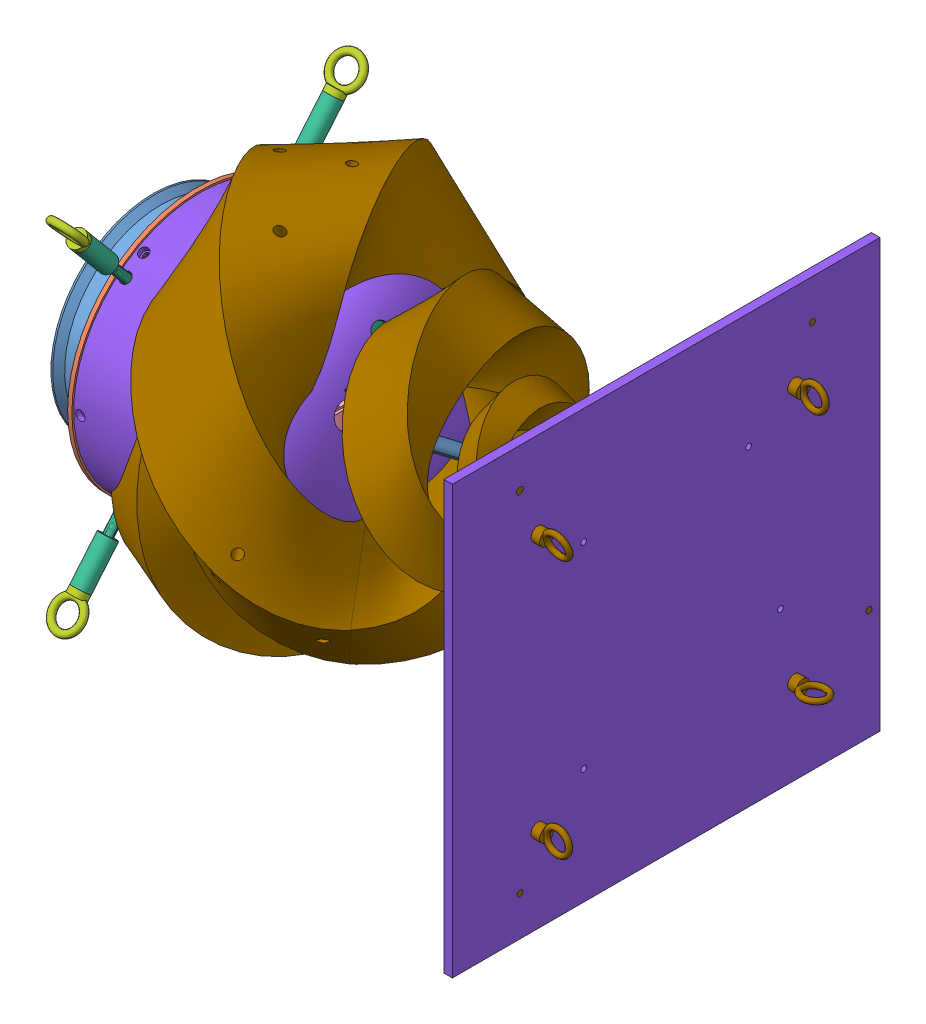
SolidWorks assembly FMアセンブリ, configuration ﾃﾞﾌｫﾙﾄ. Lengths in mm.
Overall size (642.93 538.29 530.19).
78 component instances, 31 part files, 153 mates.
Components (placement in the parent):
- PAF_interface_frame-1: PAF_interface_frame [ﾃﾞﾌｫﾙﾄ] at (23.1546 0 0) x (0 0.382683 0.92388) z (0 0.92388 -0.382683) size (272 50 272)
- Base_Plate2-1: Base_Plate2 [ﾃﾞﾌｫﾙﾄ] at (50 0 0) x (0 0 -1) z (1 0 0) size (300 300 21)
- 電池固定部材_BOTTOM-1: 電池固定部材_BOTTOM [Default] at (71 0 0) x (0 -1 0) z (0 0 1) size (277.98 10 278)
- Main_Pipe2-1: Main_Pipe2 [Default] at (71 0 0) x (0 1 0) z (0 0 -1) size (116.57 150 120)
- Battery-1: Battery [Default] at (76 0 -102.3) x (0 0 1) z (0 1 0) size (69 119 35.6)
- Battery-2: Battery [Default] at (76 -44.3863 -92.1691) x (0 0.433884 0.900969) z (0 0.900969 -0.433884) size (69 119 35.6)
- Battery-3: Battery [Default] at (76 -79.9814 -63.783) x (0 0.781831 0.62349) z (0 0.62349 -0.781831) size (69 119 35.6)
- Battery-4: Battery [Default] at (76 -99.7351 -22.7639) x (0 0.974928 0.222521) z (0 0.222521 -0.974928) size (69 119 35.6)
- Battery-5: Battery [Default] at (76 -99.7351 22.7639) x (0 0.974928 -0.222521) z (0 -0.222521 -0.974928) size (69 119 35.6)
- Battery-6: Battery [Default] at (76 -79.9814 63.783) x (0 0.781831 -0.62349) z (0 -0.62349 -0.781831) size (69 119 35.6)
- Battery-7: Battery [Default] at (76 -44.3863 92.1691) x (0 0.433884 -0.900969) z (0 -0.900969 -0.433884) size (69 119 35.6)
- Battery-8: Battery [Default] at (76 0 102.3) x (0 0 -1) z (0 -1 0) size (69 119 35.6)
- Battery-9: Battery [Default] at (76 44.3863 92.1691) x (0 -0.433884 -0.900969) z (0 -0.900969 0.433884) size (69 119 35.6)
- Battery-10: Battery [Default] at (76 79.9814 63.783) x (0 -0.781831 -0.62349) z (0 -0.62349 0.781831) size (69 119 35.6)
- Battery-11: Battery [Default] at (76 99.7351 22.7639) x (0 -0.974928 -0.222521) z (0 -0.222521 0.974928) size (69 119 35.6)
- Battery-12: Battery [Default] at (76 99.7351 -22.7639) x (0 -0.974928 0.222521) z (0 0.222521 0.974928) size (69 119 35.6)
- Battery-13: Battery [Default] at (76 79.9814 -63.783) x (0 -0.781831 0.62349) z (0 0.62349 0.781831) size (69 119 35.6)
- Battery-14: Battery [Default] at (76 44.3863 -92.1691) x (0 -0.433884 0.900969) z (0 0.900969 0.433884) size (69 119 35.6)
- 電池固定部材_TOP-1: 電池固定部材_TOP [Default] at (191 0 0) x (0 1 0) z (0 0 -1) size (277.98 10 278)
- M3×25スペーサー-1: M3×25スペーサー [Default] at (226 31.6228 45) x (0 1 0) z (0 0 1) size (6.35 31 5.5)
- M3×25スペーサー-2: M3×25スペーサー [Default] at (226 -31.6228 -45) x (0 0.996783 0.08015) z (0 -0.08015 0.996783) size (6.35 31 5.5)
- M3×25スペーサー-3: M3×25スペーサー [Default] at (226 31.6228 -45) x (0 0.39206 -0.919939) z (0 0.919939 0.39206) size (6.35 31 5.5)
- M3×25スペーサー-4: M3×25スペーサー [Default] at (226 -31.6228 45) x (0 0.187799 -0.982207) z (0 0.982207 0.187799) size (6.35 31 5.5)
- cover-1: cover [ﾃﾞﾌｫﾙﾄ] at (15 0 0) x (0 0.993404 0.114665) z (1 0 0) size (296 296 250)
- uzumaki_ver4.7_4-1: uzumaki_ver4.7_4 [ﾃﾞﾌｫﾙﾄ] at (15 0 0) x (0 0.993404 0.114665) z (1 0 0) size (487.44 471.45 440.07)
- stay1-1: stay1 [ﾃﾞﾌｫﾙﾄ] at (13.0973 5.3852 14.4171) x (0.024022 0.848578 0.528524) z (0.993238 0.039807 -0.109056) size (67.26 20.25 187.71)
- Dsub_9pin-1: Dsub_9pin [ﾃﾞﾌｫﾙﾄ] at (274.5425 31.7639 -104.6722) x (0.172763 -0.984526 -0.029346) z (0.830723 0.161653 -0.532698) size (30.8 12.6 17.3)
- M2.6×2中空スペーサー-1: M2.6×2中空スペーサー [ﾃﾞﾌｫﾙﾄ] at (275.0421 44.5828 -106.0102) x (0.549747 -0.087616 0.830723) z (-0.830723 -0.161653 0.532698) size (5 5 2)
- M2.6×2中空スペーサー-2: M2.6×2中空スペーサー [ﾃﾞﾌｫﾙﾄ] at (279.3595 19.9795 -106.7436) x (-0.227468 -0.774811 -0.589853) z (-0.830723 -0.161653 0.532698) size (5 5 2)
- M2.6×15CAP-1: M2.6×15CAP [ﾃﾞﾌｫﾙﾄ] at (270.307 43.6614 -102.9738) x (0.473537 0.297901 0.828865) z (0.830723 0.161653 -0.532698) size (4.5 4.5 17.5)
- M2.6×15CAP-2: M2.6×15CAP [ﾃﾞﾌｫﾙﾄ] at (274.6244 19.0581 -103.7072) x (0.394559 0.504073 0.768267) z (0.830723 0.161653 -0.532698) size (4.5 4.5 17.5)
- M2.5ナット-1: M2.5ナット [ﾃﾞﾌｫﾙﾄ] at (284.1831 20.9182 -109.8367) x (-0.39921 -0.49393 -0.772441) z (-0.830723 -0.161653 0.532698) size (5.1 5.77 2)
- M2.5ナット-2: M2.5ナット [ﾃﾞﾌｫﾙﾄ] at (279.8658 45.5215 -109.1034) x (0.546065 -0.050599 0.836214) z (-0.830723 -0.161653 0.532698) size (5.1 5.77 2)
- Dsub_9pin_オス-1: Dsub_9pin_オス [ﾃﾞﾌｫﾙﾄ] at (280.363 32.8965 -108.4046) x (-0.172763 0.984526 0.029346) z (-0.830723 -0.161653 0.532698) size (30.8 12.6 17.3)
- U1F-72-818-1: U1F-72-818 [ﾃﾞﾌｫﾙﾄ] at (50 0 0) x (0 0 1) z (-1 0 0) size (102 50 3.5)
- U1F-72-819-1: U1F-72-819 [ﾃﾞﾌｫﾙﾄ] at (46.5 0 0) x (0 0.866025 0.5) z (-1 0 0) size (46.37 40.16 29.2)
- U1F-72-820-2: U1F-72-820 [ﾃﾞﾌｫﾙﾄ] at (17.3 14 0) x (0 -1 0) z (-1 0 0) size (40 20 20)
- U1F-72-820-3: U1F-72-820 [ﾃﾞﾌｫﾙﾄ] at (17.3 -7 -12.1244) x (0 0.5 0.866025) z (-1 0 0) size (40 20 20)
- U1F-72-820-4: U1F-72-820 [ﾃﾞﾌｫﾙﾄ] at (17.3 -7 12.1244) x (0 0.5 -0.866025) z (-1 0 0) size (40 20 20)
- switch-1: switch [ﾃﾞﾌｫﾙﾄ] at (13.15 44.34 -0.05) x (0 1 0) z (-1 0 0) size (20.4 6.5 19.83)
- switch-2: switch [ﾃﾞﾌｫﾙﾄ] at (13.15 -22.2133 -38.3746) x (0 -0.5 -0.866025) z (-1 0 0) size (20.4 6.5 19.83)
- switch-3: switch [ﾃﾞﾌｫﾙﾄ] at (13.15 -22.2133 38.3746) x (0 -0.5 0.866025) z (-1 0 0) size (20.4 6.5 19.83)
- OBC-1: OBC [ﾃﾞﾌｫﾙﾄ] at (153 -14.7214 0) x (1 0 0) z (0 -1 0) size (150 70 11.6)
- M3×5_スペーサー-1: M3×5_スペーサー [ﾃﾞﾌｫﾙﾄ] at (210 -14.7214 30) x (1 0 0) z (0 1 0) size (6 6 5)
- M3×5_スペーサー-2: M3×5_スペーサー [ﾃﾞﾌｫﾙﾄ] at (210 -14.7214 -30) x (1 0 0) z (0 1 0) size (6 6 5)
- M3×5_スペーサー-3: M3×5_スペーサー [ﾃﾞﾌｫﾙﾄ] at (101 -14.7214 17.5) x (1 0 0) z (0 1 0) size (6 6 5)
- M3×5_スペーサー-4: M3×5_スペーサー [ﾃﾞﾌｫﾙﾄ] at (96 -14.7214 -30) x (1 0 0) z (0 1 0) size (6 6 5)
- 送信機-1: 送信機 [Default] at (158 9.7214 0) size (120 16.5 42)
- 電磁シールド-1: 電磁シールド [ﾃﾞﾌｫﾙﾄ] at (223 9.7214 0) x (0 1 0) z (-1 0 0) size (31 70 130)
- 吊り上げ冶具_LONG-1: 吊り上げ冶具_LONG [ﾃﾞﾌｫﾙﾄ] at (63 91.9253 77.1345) x (1 0 0) z (0 0.766044 0.642788) size (20 20 110)
- 吊り上げ冶具_LONG-2: 吊り上げ冶具_LONG [ﾃﾞﾌｫﾙﾄ] at (63 -91.9253 77.1345) x (1 0 0) z (0 -0.766044 0.642788) size (20 20 110)
- 吊り上げ冶具_LONG-3: 吊り上げ冶具_LONG [ﾃﾞﾌｫﾙﾄ] at (63 -54.4789 -106.9208) x (1 0 0) z (0 -0.45399 -0.891007) size (20 20 110)
- 吊り上げ冶具_LONG-4: 吊り上げ冶具_LONG [ﾃﾞﾌｫﾙﾄ] at (63 91.9253 -77.1345) x (1 0 0) z (0 0.766044 -0.642788) size (20 20 110)
- M10アイボルト-5: M10アイボルト [ﾃﾞﾌｫﾙﾄ] at (63 -162.4014 136.271) x (0.031652 -0.642466 -0.765661) z (0 -0.766044 0.642788) size (20 41 62)
- M10アイボルト-6: M10アイボルト [ﾃﾞﾌｫﾙﾄ] at (63 -96.246 -188.8934) x (-0.000192 0.891007 -0.45399) z (0 -0.45399 -0.891007) size (20 41 62)
- M10アイボルト-7: M10アイボルト [ﾃﾞﾌｫﾙﾄ] at (63 162.4014 -136.271) x (0.071151 0.641158 0.764103) z (0 0.766044 -0.642788) size (20 41 62)
- M10アイボルト-8: M10アイボルト [ﾃﾞﾌｫﾙﾄ] at (63 162.4014 136.271) x (0 -0.642788 0.766044) z (0 0.766044 0.642788) size (20 41 62)
- 吊り上げ冶具TOP-1: 吊り上げ冶具TOP [ﾃﾞﾌｫﾙﾄ] at (600 0 0) x (0 0 1) z (-1 0 0) size (500 500 10)
- M8アイボルト-1: M8アイボルト [ﾃﾞﾌｫﾙﾄ] at (600 203.7678 -170.9815) x (0 0 1) z (-1 0 0) size (16 32.6 49.45)
- M8アイボルト-2: M8アイボルト [ﾃﾞﾌｫﾙﾄ] at (600 -120.7615 -237.0077) x (0 0 1) z (-1 0 0) size (16 32.6 49.45)
- M8アイボルト-3: M8アイボルト [ﾃﾞﾌｫﾙﾄ] at (600 203.7678 170.9815) x (0 0.963199 0.26879) z (-1 0 0) size (16 32.6 49.45)
- M8アイボルト-4: M8アイボルト [ﾃﾞﾌｫﾙﾄ] at (600 -203.7678 170.9815) x (0 0 1) z (-1 0 0) size (16 32.6 49.45)
- M8アイボルト-5: M8アイボルト [ﾃﾞﾌｫﾙﾄ] at (590 150 150) x (0 0.249704 -0.968322) z (1 0 0) size (16 32.6 49.45)
- M8アイボルト-6: M8アイボルト [ﾃﾞﾌｫﾙﾄ] at (590 150 -150) x (0 0 -1) z (1 0 0) size (16 32.6 49.45)
- M8アイボルト-7: M8アイボルト [ﾃﾞﾌｫﾙﾄ] at (590 -150 150) x (0 0 -1) z (1 0 0) size (16 32.6 49.45)
- M8アイボルト-8: M8アイボルト [ﾃﾞﾌｫﾙﾄ] at (590 -150 -150) x (0 0.99163 -0.129116) z (1 0 0) size (16 32.6 49.45)
- Supporting_pole-1: Supporting_pole [Default] at (71 81.0537 101.6381) x (0 -1 0) z (0 0 1) size (10 125 10)
- Supporting_pole-2: Supporting_pole [Default] at (196 130 0) x (0 0.996899 0.07869) z (0 -0.07869 0.996899) size (10 125 10)
- Supporting_pole-3: Supporting_pole [Default] at (196 81.0537 -101.6381) x (0 0.918275 0.395944) z (0 -0.395944 0.918275) size (10 125 10)
- Supporting_pole-4: Supporting_pole [Default] at (71 -81.0537 -101.6381) x (0 -1 0) z (0 0 1) size (10 125 10)
- Supporting_pole-5: Supporting_pole [Default] at (71 -130 0) x (0 -1 0) z (0 0 1) size (10 125 10)
- Supporting_pole-6: Supporting_pole [Default] at (71 -81.0537 101.6381) x (0 -0.991414 0.130764) z (0 0.130764 0.991414) size (10 125 10)
- ハブ基板-1: ハブ基板 [Default] at (235 0 0) x (0 1 0) z (0 0 1) size (206.28 45.66 208.72)
- M3×12CAP-1: M3×12CAP [ﾃﾞﾌｫﾙﾄ] at (238 -31.6228 -45) x (0 0 1) z (-1 0 0) size (5.5 5.5 15)
- M3×12CAP-2: M3×12CAP [ﾃﾞﾌｫﾙﾄ] at (238 31.6228 -45) x (0 0 1) z (-1 0 0) size (5.5 5.5 15)
- M3×12CAP-3: M3×12CAP [ﾃﾞﾌｫﾙﾄ] at (238 31.6228 45) x (0 0 1) z (-1 0 0) size (5.5 5.5 15)
- M3×12CAP-4: M3×12CAP [ﾃﾞﾌｫﾙﾄ] at (238 -31.6228 45) x (0 0 1) z (-1 0 0) size (5.5 5.5 15)
- hub_insulator-1: hub_insulator [ﾃﾞﾌｫﾙﾄ] at (232 -0.0001 -0.0001) x (0 -1 -0.000003) z (-1 0 0) size (140 140 6.04)
Mates (geometry in assembly coordinates):
- 一致3: coincident: line of PAF_interface_frame-1 through (123.9718 0 0) axis (-1 0 0); point of assembly
- 一致4: coincident anti-aligned: plane of PAF_interface_frame-1 through (0 -45.7307 -110.4036) normal (-1 0 0); plane of assembly through (0 0 0) normal (1 0 0)
- 一致5: coincident anti-aligned: plane of PAF_interface_frame-1 through (50 -41.9038 -101.1648) normal (1 0 0); plane of Base_Plate2-1 through (50 0 0) normal (-1 0 0)
- 同心円1: concentric anti-aligned: cylinder of PAF_interface_frame-1 through (58.3329 0 0) axis (1 0 0) radius 136; cylinder of Base_Plate2-1 through (71 0 0) axis (-1 0 0) radius 140
- 平行1: parallel anti-aligned: plane of Base_Plate2-1 through (71 -25 -20) normal (0 -1 0); plane of assembly through (0 0 0) normal (0 1 0)
- 同心円2: concentric aligned: cylinder of PAF_interface_frame-1 through (50 113.6372 47.0701) axis (-1 0 0) radius 3.3; cylinder of Base_Plate2-1 through (50 113.6372 47.0701) axis (-1 0 0) radius 2.5
- 一致7: coincident anti-aligned: plane of Base_Plate2-1 through (71 0 0) normal (1 0 0); plane of 電池固定部材_BOTTOM-1 through (71 0 0) normal (-1 0 0)
- 同心円3: concentric aligned: cylinder of Base_Plate2-1 through (71 0 0) axis (-1 0 0) radius 140; cylinder of 電池固定部材_BOTTOM-1 through (81 0 0) axis (-1 0 0) radius 139
- 同心円4: concentric anti-aligned: cylinder of Base_Plate2-1 through (50 130 0) axis (-1 0 0) radius 2.9; cylinder of 電池固定部材_BOTTOM-1 through (71 130 0) axis (1 0 0) radius 5.1
- 一致8: coincident anti-aligned: plane of Base_Plate2-1 through (71 0 0) normal (1 0 0); plane of Main_Pipe2-1 through (71 0 0) normal (-1 0 0)
- 同心円5: concentric aligned: cylinder of 電池固定部材_BOTTOM-1 through (81 0 0) axis (-1 0 0) radius 61; cylinder of Main_Pipe2-1 through (221 0 0) axis (-1 0 0) radius 60
- 同心円6: concentric aligned: cylinder of Base_Plate2-1 through (71 40 0) axis (-1 0 0) radius 15; cylinder of Main_Pipe2-1 through (221 40 0) axis (-1 0 0) radius 15
- 一致9: coincident anti-aligned: plane of 電池固定部材_BOTTOM-1 through (76 0 119) normal (1 0 0); plane of Battery-1 through (76 0 -119) normal (-1 0 0)
- 平行3: parallel anti-aligned: plane of 電池固定部材_BOTTOM-1 through (76 -18.5 -119) normal (0 1 0); plane of Battery-1 through (195 -17.8 -119) normal (0 -1 0)
- 同心円9: concentric anti-aligned: cylinder of 電池固定部材_BOTTOM-1 through (76 0 -119) axis (1 0 0) radius 18.5; cylinder of Battery-1 through (195 0 -119) axis (-1 0 0) radius 17.8
- 同心円10: concentric anti-aligned: cylinder of Main_Pipe2-1 through (199 0 0) axis (1 0 0) radius 50; cylinder of 電池固定部材_TOP-1 through (199 0 0) axis (-1 0 0) radius 60
- 平行4: parallel anti-aligned: plane of Battery-11 through (195 119.9773 9.1263) normal (0 0.222521 -0.974928); plane of 電池固定部材_TOP-1 through (199 120.1331 8.4438) normal (0 -0.222521 0.974928)
- 一致14: coincident anti-aligned: plane of Main_Pipe2-1 through (199 0 0) normal (1 0 0); plane of 電池固定部材_TOP-1 through (199 0 0) normal (-1 0 0)
- 同心円11: concentric aligned: cylinder of Main_Pipe2-1 through (199 -31.6228 45) axis (1 0 0) radius 1.25; cylinder of M3×25スペーサー-4 through (195 -31.6228 45) axis (1 0 0) radius 1.5
- 同心円12: concentric anti-aligned: cylinder of Main_Pipe2-1 through (199 -31.6228 -45) axis (1 0 0) radius 1.25; circle of M3×25スペーサー-2
- 同心円13: concentric aligned: cylinder of Main_Pipe2-1 through (199 31.6228 -45) axis (1 0 0) radius 1.25; cylinder of M3×25スペーサー-3 through (195 31.6228 -45) axis (1 0 0) radius 1.5
- 同心円14: concentric aligned: cylinder of Main_Pipe2-1 through (199 31.6228 45) axis (1 0 0) radius 1.25; cylinder of M3×25スペーサー-1 through (195 31.6228 45) axis (1 0 0) radius 1.5
- 一致15: coincident anti-aligned: plane of 電池固定部材_TOP-1 through (201 0 0) normal (1 0 0); plane of M3×25スペーサー-1 through (201 31.6228 45) normal (-1 0 0)
- 一致16: coincident anti-aligned: plane of 電池固定部材_TOP-1 through (201 0 0) normal (1 0 0); plane of M3×25スペーサー-2 through (201 -31.6228 -45) normal (-1 0 0)
- 一致17: coincident anti-aligned: plane of 電池固定部材_TOP-1 through (201 0 0) normal (1 0 0); plane of M3×25スペーサー-4 through (201 -31.6228 45) normal (-1 0 0)
- 一致18: coincident anti-aligned: plane of 電池固定部材_TOP-1 through (201 0 0) normal (1 0 0); plane of M3×25スペーサー-3 through (201 31.6228 -45) normal (-1 0 0)
- 同心円17: concentric anti-aligned: cylinder of Base_Plate2-1 through (71 0 0) axis (-1 0 0) radius 140; cylinder of cover-1 through (569.0392 0 0) axis (1 0 0) radius 145
- 同心円18: concentric aligned: cylinder of cover-1 through (569.0392 0 0) axis (1 0 0) radius 148; cylinder of uzumaki_ver4.7_4-1 through (569.0392 0 0) axis (1 0 0) radius 148
- 同心円19: concentric aligned: cylinder of cover-1 through (167.9289 -257.7357 233.8296) axis (0 -0.74062 0.671924) radius 3.5; cylinder of uzumaki_ver4.7_4-1 through (167.9289 -257.7357 233.8296) axis (0 -0.74062 0.671924) radius 5.5
- 同心円20: concentric aligned: cylinder of Base_Plate2-1 through (63 0 -140) axis (0 0 -1) radius 2.5; cylinder of cover-1 through (63 0 -148) axis (0 0 -1) radius 5.5
- 一致30: coincident anti-aligned: plane of uzumaki_ver4.7_4-1 through (483.5975 94.0469 35.0545) normal (-0.966676 -0.253899 -0.03274); plane of stay1-1 through (483.5975 94.0469 35.0545) normal (0.966676 0.253899 0.03274)
- 同心円33: concentric aligned: cylinder of uzumaki_ver4.7_4-1 through (435.2636 81.352 33.4176) axis (0.966676 0.253899 0.03274) radius 7.5; cylinder of stay1-1 through (-499986.9199 -131355.3348 -16915.0779) axis (0.966676 0.253899 0.03274) radius 7.5
- 同心円34: concentric aligned: cylinder of cover-1 through (285.0108 46.5227 -112.4026) axis (0.830723 0.161653 -0.532698) radius 1.525; cylinder of Dsub_9pin-1 through (273.3807 44.2595 -104.9448) axis (0.830723 0.161653 -0.532698) radius 1.524
- 一致32: coincident anti-aligned: plane of Base_Plate2-1 through (50 0 0) normal (-1 0 0); plane of U1F-72-818-1 through (50 0 0) normal (1 0 0)
- 同心円39: concentric aligned: cylinder of Base_Plate2-1 through (50 -16 0) axis (-1 0 0) radius 1.65; cylinder of U1F-72-818-1 through (46.5 -16 0) axis (-1 0 0) radius 4
- 同心円40: concentric aligned: cylinder of Base_Plate2-1 through (50 -16 42) axis (-1 0 0) radius 1.65; cylinder of U1F-72-818-1 through (46.5 -16 42) axis (-1 0 0) radius 2.25
- 一致33: coincident anti-aligned: plane of U1F-72-818-1 through (46.5 0 0) normal (-1 0 0); plane of U1F-72-819-1 through (46.5 0 0) normal (1 0 0)
- 同心円41: concentric aligned: cylinder of U1F-72-818-1 through (50 0 0) axis (1 0 0) radius 2.25; cylinder of U1F-72-819-1 through (46.5 0 0) axis (1 0 0) radius 1.65
- 同心円42: concentric aligned: cylinder of U1F-72-818-1 through (50 17 0) axis (1 0 0) radius 2.25; cylinder of U1F-72-819-1 through (46.5 17 0) axis (1 0 0) radius 1.65
- 一致35: coincident anti-aligned: plane of U1F-72-819-1 through (17.3 0 0) normal (-1 0 0); plane of U1F-72-820-3 through (17.3 -7 -12.1244) normal (1 0 0)
- 同心円43: concentric aligned: cylinder of U1F-72-819-1 through (17.3 -3.8038 -18.5885) axis (-1 0 0) radius 1.25; cylinder of U1F-72-820-3 through (13.3 -3.8038 -18.5885) axis (-1 0 0) radius 3.3
- 同心円44: concentric aligned: cylinder of U1F-72-819-1 through (17.3 -14.1962 -12.5885) axis (-1 0 0) radius 1.25; cylinder of U1F-72-820-3 through (13.3 -14.1962 -12.5885) axis (-1 0 0) radius 3.3
- 一致36: coincident anti-aligned: plane of U1F-72-819-1 through (17.3 0 0) normal (-1 0 0); plane of U1F-72-820-2 through (17.3 14 0) normal (1 0 0)
- 同心円45: concentric aligned: cylinder of U1F-72-819-1 through (17.3 18 -6) axis (-1 0 0) radius 1.25; cylinder of U1F-72-820-2 through (13.3 18 -6) axis (-1 0 0) radius 3.3
- 同心円46: concentric aligned: cylinder of U1F-72-819-1 through (17.3 18 6) axis (-1 0 0) radius 1.25; cylinder of U1F-72-820-2 through (13.3 18 6) axis (-1 0 0) radius 3.3
- 一致37: coincident anti-aligned: plane of U1F-72-819-1 through (17.3 0 0) normal (-1 0 0); plane of U1F-72-820-4 through (17.3 -7 12.1244) normal (1 0 0)
- 同心円47: concentric aligned: cylinder of U1F-72-819-1 through (17.3 -3.8038 18.5885) axis (-1 0 0) radius 1.25; cylinder of U1F-72-820-4 through (13.3 -3.8038 18.5885) axis (-1 0 0) radius 3.3
- 同心円48: concentric aligned: cylinder of U1F-72-819-1 through (17.3 -14.1962 12.5885) axis (-1 0 0) radius 1.25; cylinder of U1F-72-820-4 through (13.3 -14.1962 12.5885) axis (-1 0 0) radius 3.3
- 同心円51: concentric anti-aligned: cylinder of U1F-72-820-2 through (10.8 39.5 10) axis (0 0 -1) radius 1.25; cylinder of switch-1 through (10.8 39.5 3.2) axis (0 0 1) radius 1.125
- 平行5: parallel aligned: plane of U1F-72-820-2 through (8.3 54 5.2) normal (-1 0 0); plane of switch-1 through (4.15 44.34 -0.05) normal (-1 0 0)
- 一致39: coincident anti-aligned: plane of U1F-72-820-2 through (17.3 14 3.2) normal (0 0 -1); plane of switch-1 through (4.15 34.34 3.2) normal (0 0 1)
- 同心円54: concentric anti-aligned: cylinder of U1F-72-820-4 through (10.8 -28.4103 29.208) axis (0 0.866025 0.5) radius 1.25; cylinder of switch-3 through (10.8 -22.6079 32.558) axis (0 -0.866025 -0.5) radius 1.125
- 平行7: parallel aligned: plane of U1F-72-820-4 through (8.3 -31.5033 44.1654) normal (-1 0 0); plane of switch-3 through (4.15 -22.2133 38.3746) normal (-1 0 0)
- 一致43: coincident anti-aligned: plane of U1F-72-820-4 through (17.3 -4.2287 13.7244) normal (0 -0.866025 -0.5); plane of switch-3 through (4.15 -14.3987 31.3393) normal (0 0.866025 0.5)
- 同心円55: concentric anti-aligned: cylinder of U1F-72-820-3 through (10.8 -11.0897 -39.208) axis (0 -0.866025 0.5) radius 1.25; cylinder of switch-2 through (10.8 -16.9787 -35.808) axis (0 0.866025 -0.5) radius 1.125
- 一致44: coincident anti-aligned: plane of U1F-72-820-3 through (17.3 -4.2287 -13.7244) normal (0 -0.866025 0.5); plane of switch-2 through (4.15 -14.3987 -31.3393) normal (0 0.866025 -0.5)
- 平行8: parallel aligned: plane of U1F-72-820-3 through (8.3 -29.7713 -45.1654) normal (-1 0 0); plane of switch-2 through (4.15 -22.2133 -38.3746) normal (-1 0 0)
- 一致45: coincident anti-aligned: plane of Main_Pipe2-1 through (76 -9.7214 40) normal (0 -1 0); plane of M3×5_スペーサー-1 through (210 -9.7214 30) normal (0 1 0)
- 同心円56: concentric aligned: cylinder of Main_Pipe2-1 through (210 -9.7214 30) axis (0 -1 0) radius 1.25; cylinder of M3×5_スペーサー-1 through (210 -9.7214 30) axis (0 -1 0) radius 1.5
- 一致46: coincident anti-aligned: plane of Main_Pipe2-1 through (76 -9.7214 40) normal (0 -1 0); plane of M3×5_スペーサー-2 through (210 -9.7214 -30) normal (0 1 0)
- 同心円57: concentric aligned: cylinder of Main_Pipe2-1 through (210 -9.7214 -30) axis (0 -1 0) radius 1.25; cylinder of M3×5_スペーサー-2 through (210 -9.7214 -30) axis (0 -1 0) radius 1.5
- 一致47: coincident anti-aligned: plane of Main_Pipe2-1 through (76 -9.7214 40) normal (0 -1 0); plane of M3×5_スペーサー-4 through (96 -9.7214 -30) normal (0 1 0)
- 同心円58: concentric aligned: cylinder of Main_Pipe2-1 through (96 -9.7214 -30) axis (0 -1 0) radius 1.25; cylinder of M3×5_スペーサー-4 through (96 -9.7214 -30) axis (0 -1 0) radius 1.5
- 一致48: coincident anti-aligned: plane of Main_Pipe2-1 through (76 -9.7214 40) normal (0 -1 0); plane of M3×5_スペーサー-3 through (101 -9.7214 17.5) normal (0 1 0)
- 同心円59: concentric anti-aligned: cylinder of Main_Pipe2-1 through (101 9.7214 17.5) axis (0 1 0) radius 1.25; cylinder of M3×5_スペーサー-3 through (101 -9.7214 17.5) axis (0 -1 0) radius 1.5
- 一致49: coincident anti-aligned: plane of OBC-1 through (153 -14.7214 0) normal (0 1 0); plane of M3×5_スペーサー-2 through (210 -14.7214 -30) normal (0 -1 0)
- 同心円60: concentric aligned: cylinder of OBC-1 through (210 -16.3214 -30) axis (0 -1 0) radius 1.8; cylinder of M3×5_スペーサー-2 through (210 -9.7214 -30) axis (0 -1 0) radius 1.5
- 同心円61: concentric aligned: cylinder of OBC-1 through (210 -16.3214 30) axis (0 -1 0) radius 1.8; cylinder of M3×5_スペーサー-1 through (210 -9.7214 30) axis (0 -1 0) radius 1.5
- 一致50: coincident anti-aligned: plane of Main_Pipe2-1 through (76 9.7214 40) normal (0 1 0); plane of 送信機-1 through (158 9.7214 0) normal (0 -1 0)
- 同心円62: concentric aligned: cylinder of Main_Pipe2-1 through (215 9.7214 0) axis (0 1 0) radius 1.25; cylinder of 送信機-1 through (215 11.7214 0) axis (0 1 0) radius 1.8
- 同心円63: concentric aligned: cylinder of Main_Pipe2-1 through (215 9.7214 17.5) axis (0 1 0) radius 1.25; cylinder of 送信機-1 through (215 11.7214 17.5) axis (0 1 0) radius 1.8
- 一致51: coincident anti-aligned: plane of Main_Pipe2-1 through (76 9.7214 40) normal (0 1 0); plane of 電磁シールド-1 through (93 9.7214 -35) normal (0 -1 0)
- 同心円64: concentric aligned: cylinder of Main_Pipe2-1 through (198 9.7214 30) axis (0 1 0) radius 1.25; cylinder of 電磁シールド-1 through (198 10.7214 30) axis (0 1 0) radius 1.6
- 同心円65: concentric aligned: cylinder of Main_Pipe2-1 through (198 9.7214 -30) axis (0 1 0) radius 1.25; cylinder of 電磁シールド-1 through (198 10.7214 -30) axis (0 1 0) radius 1.6
- 同心円66: concentric anti-aligned: cylinder of 吊り上げ冶具_LONG-1 through (63 137.888 115.7018) axis (0 -0.766044 -0.642788) radius 5; cylinder of cover-1 through (63 113.3746 95.1326) axis (0 0.766044 0.642788) radius 6
- 一致53: coincident: point of Base_Plate2-1; point of 吊り上げ冶具_LONG-1
- 同心円67: concentric anti-aligned: cylinder of Base_Plate2-1 through (63 -107.2462 89.9903) axis (0 -0.766044 0.642788) radius 4.5; cylinder of 吊り上げ冶具_LONG-2 through (63 -137.888 115.7018) axis (0 0.766044 -0.642788) radius 5
- 一致55: coincident: point of Base_Plate2-1; point of 吊り上げ冶具_LONG-2
- 同心円68: concentric anti-aligned: cylinder of Base_Plate2-1 through (63 -63.5587 -124.7409) axis (0 -0.45399 -0.891007) radius 4.5; cylinder of 吊り上げ冶具_LONG-3 through (63 -81.7183 -160.3812) axis (0 0.45399 0.891007) radius 5
- 一致56: coincident: point of Base_Plate2-1; point of 吊り上げ冶具_LONG-3
- 同心円69: concentric anti-aligned: cylinder of Base_Plate2-1 through (63 107.2462 -89.9903) axis (0 0.766044 -0.642788) radius 4.5; cylinder of 吊り上げ冶具_LONG-4 through (63 137.888 -115.7018) axis (0 -0.766044 0.642788) radius 5
- 一致57: coincident: point of Base_Plate2-1; point of 吊り上げ冶具_LONG-4
- 同心円83: concentric anti-aligned: cylinder of 吊り上げ冶具_LONG-2 through (63 -176.1902 147.8412) axis (0 -0.766044 0.642788) radius 4.25; cylinder of M10アイボルト-5 through (63 -181.5525 152.3407) axis (0 0.766044 -0.642788) radius 5
- 一致71: coincident anti-aligned: plane of 吊り上げ冶具_LONG-2 through (63 -176.1902 147.8412) normal (0 -0.766044 0.642788); plane of M10アイボルト-5 through (63 -176.1902 147.8412) normal (0 0.766044 -0.642788)
- 同心円84: concentric anti-aligned: cylinder of 吊り上げ冶具_LONG-3 through (63 -104.4178 -204.9315) axis (0 -0.45399 -0.891007) radius 4.25; cylinder of M10アイボルト-6 through (63 -107.5957 -211.1685) axis (0 0.45399 0.891007) radius 5
- 一致72: coincident anti-aligned: plane of 吊り上げ冶具_LONG-3 through (63 -104.4178 -204.9315) normal (0 -0.45399 -0.891007); plane of M10アイボルト-6 through (63 -104.4178 -204.9315) normal (0 0.45399 0.891007)
- 同心円85: concentric anti-aligned: cylinder of 吊り上げ冶具_LONG-4 through (63 176.1902 -147.8412) axis (0 0.766044 -0.642788) radius 4.25; cylinder of M10アイボルト-7 through (63 181.5525 -152.3407) axis (0 -0.766044 0.642788) radius 5
- 一致73: coincident anti-aligned: plane of 吊り上げ冶具_LONG-4 through (63 176.1902 -147.8412) normal (0 0.766044 -0.642788); plane of M10アイボルト-7 through (63 176.1902 -147.8412) normal (0 -0.766044 0.642788)
- 同心円86: concentric anti-aligned: cylinder of 吊り上げ冶具_LONG-1 through (63 176.1902 147.8412) axis (0 0.766044 0.642788) radius 4.25; cylinder of M10アイボルト-8 through (63 181.5525 152.3407) axis (0 -0.766044 -0.642788) radius 5
- 一致74: coincident anti-aligned: plane of 吊り上げ冶具_LONG-1 through (63 176.1902 147.8412) normal (0 0.766044 0.642788); plane of M10アイボルト-8 through (63 176.1902 147.8412) normal (0 -0.766044 -0.642788)
- 距離1: distance = 600 mm aligned: plane of assembly through (0 0 0) normal (1 0 0); plane of 吊り上げ冶具TOP-1 through (600 0 0) normal (1 0 0)
- 一致82: coincident aligned: line of PAF_interface_frame-1 through (123.9718 0 0) axis (-1 0 0); line of 吊り上げ冶具TOP-1 through (701.7257 0 0) axis (-1 0 0)
- 平行9: parallel aligned: plane of 吊り上げ冶具TOP-1 through (590 250 -250) normal (0 1 0); plane of assembly through (0 0 0) normal (0 1 0)
- 同心円97: concentric anti-aligned: cylinder of M8アイボルト-1 through (580 203.7678 -170.9815) axis (1 0 0) radius 4; cylinder of 吊り上げ冶具TOP-1 through (590 203.7678 -170.9815) axis (-1 0 0) radius 3.4
- 一致84: coincident anti-aligned: plane of 吊り上げ冶具TOP-1 through (590 0 0) normal (-1 0 0); plane of M8アイボルト-1 through (590 203.7678 -170.9815) normal (1 0 0)
- 同心円98: concentric anti-aligned: cylinder of M8アイボルト-2 through (580 -120.7615 -237.0077) axis (1 0 0) radius 4; cylinder of 吊り上げ冶具TOP-1 through (590 -120.7615 -237.0077) axis (-1 0 0) radius 3.4
- 一致85: coincident anti-aligned: plane of 吊り上げ冶具TOP-1 through (590 0 0) normal (-1 0 0); plane of M8アイボルト-2 through (590 -120.7615 -237.0077) normal (1 0 0)
- 同心円99: concentric anti-aligned: cylinder of M8アイボルト-3 through (580 203.7678 170.9815) axis (1 0 0) radius 4; cylinder of 吊り上げ冶具TOP-1 through (590 203.7678 170.9815) axis (-1 0 0) radius 3.4
- 一致86: coincident anti-aligned: plane of 吊り上げ冶具TOP-1 through (590 0 0) normal (-1 0 0); plane of M8アイボルト-3 through (590 203.7678 170.9815) normal (1 0 0)
- 同心円100: concentric anti-aligned: cylinder of M8アイボルト-4 through (580 -203.7678 170.9815) axis (1 0 0) radius 4; cylinder of 吊り上げ冶具TOP-1 through (590 -203.7678 170.9815) axis (-1 0 0) radius 3.4
- 一致87: coincident anti-aligned: plane of 吊り上げ冶具TOP-1 through (590 0 0) normal (-1 0 0); plane of M8アイボルト-4 through (590 -203.7678 170.9815) normal (1 0 0)
- 同心円101: concentric aligned: cylinder of 吊り上げ冶具TOP-1 through (590 150 150) axis (-1 0 0) radius 3.4; cylinder of M8アイボルト-5 through (610 150 150) axis (-1 0 0) radius 4
- 一致88: coincident anti-aligned: plane of 吊り上げ冶具TOP-1 through (600 0 0) normal (1 0 0); plane of M8アイボルト-5 through (600 150 150) normal (-1 0 0)
- 同心円102: concentric aligned: cylinder of 吊り上げ冶具TOP-1 through (590 150 -150) axis (-1 0 0) radius 3.4; cylinder of M8アイボルト-6 through (610 150 -150) axis (-1 0 0) radius 4
- 一致89: coincident anti-aligned: plane of 吊り上げ冶具TOP-1 through (600 0 0) normal (1 0 0); plane of M8アイボルト-6 through (600 150 -150) normal (-1 0 0)
- 同心円103: concentric aligned: cylinder of 吊り上げ冶具TOP-1 through (590 -150 150) axis (-1 0 0) radius 3.4; cylinder of M8アイボルト-7 through (610 -150 150) axis (-1 0 0) radius 4
- 一致90: coincident anti-aligned: plane of 吊り上げ冶具TOP-1 through (600 0 0) normal (1 0 0); plane of M8アイボルト-7 through (600 -150 150) normal (-1 0 0)
- 同心円104: concentric aligned: cylinder of 吊り上げ冶具TOP-1 through (590 -150 -150) axis (-1 0 0) radius 3.4; cylinder of M8アイボルト-8 through (610 -150 -150) axis (-1 0 0) radius 4
- 一致92: coincident anti-aligned: plane of 吊り上げ冶具TOP-1 through (600 0 0) normal (1 0 0); plane of M8アイボルト-8 through (600 -150 -150) normal (-1 0 0)
- 同心円105: concentric anti-aligned: cylinder of 電池固定部材_BOTTOM-1 through (71 -130 0) axis (1 0 0) radius 5.1; cylinder of Supporting_pole-5 through (196 -130 0) axis (-1 0 0) radius 5
- 一致93: coincident anti-aligned: plane of 電池固定部材_TOP-1 through (196 -130 0) normal (-1 0 0); plane of Supporting_pole-5 through (196 -130 0) normal (1 0 0)
- 同心円106: concentric anti-aligned: cylinder of 電池固定部材_BOTTOM-1 through (71 -81.0537 101.6381) axis (1 0 0) radius 5.1; cylinder of Supporting_pole-6 through (196 -81.0537 101.6381) axis (-1 0 0) radius 5
- 一致94: coincident anti-aligned: plane of 電池固定部材_TOP-1 through (196 -81.0537 101.6381) normal (-1 0 0); plane of Supporting_pole-6 through (196 -81.0537 101.6381) normal (1 0 0)
- 同心円107: concentric anti-aligned: cylinder of 電池固定部材_BOTTOM-1 through (71 81.0537 101.6381) axis (1 0 0) radius 5.1; cylinder of Supporting_pole-1 through (196 81.0537 101.6381) axis (-1 0 0) radius 5
- 一致95: coincident anti-aligned: plane of 電池固定部材_TOP-1 through (196 81.0537 101.6381) normal (-1 0 0); plane of Supporting_pole-1 through (196 81.0537 101.6381) normal (1 0 0)
- 同心円109: concentric anti-aligned: cylinder of 電池固定部材_TOP-1 through (196 130 0) axis (-1 0 0) radius 5.1; cylinder of Supporting_pole-2 through (71 130 0) axis (1 0 0) radius 5
- 一致96: coincident anti-aligned: plane of 電池固定部材_TOP-1 through (196 130 0) normal (-1 0 0); plane of Supporting_pole-2 through (196 130 0) normal (1 0 0)
- 同心円110: concentric anti-aligned: cylinder of 電池固定部材_TOP-1 through (196 81.0537 -101.6381) axis (-1 0 0) radius 5.1; cylinder of Supporting_pole-3 through (71 81.0537 -101.6381) axis (1 0 0) radius 5
- 一致97: coincident anti-aligned: plane of 電池固定部材_TOP-1 through (196 81.0537 -101.6381) normal (-1 0 0); plane of Supporting_pole-3 through (196 81.0537 -101.6381) normal (1 0 0)
- 同心円111: concentric anti-aligned: cylinder of 電池固定部材_BOTTOM-1 through (71 -81.0537 -101.6381) axis (1 0 0) radius 5.1; cylinder of Supporting_pole-4 through (196 -81.0537 -101.6381) axis (-1 0 0) radius 5
- 一致98: coincident anti-aligned: plane of 電池固定部材_TOP-1 through (196 -81.0537 -101.6381) normal (-1 0 0); plane of Supporting_pole-4 through (196 -81.0537 -101.6381) normal (1 0 0)
- 同心円114: concentric aligned: cylinder of cover-1 through (289.3282 21.9194 -113.1359) axis (0.830723 0.161653 -0.532698) radius 1.525; cylinder of Dsub_9pin-1 through (277.698 19.6562 -105.6782) axis (0.830723 0.161653 -0.532698) radius 1.524
- 同心円115: concentric aligned: cylinder of cover-1 through (285.0108 46.5227 -112.4026) axis (0.830723 0.161653 -0.532698) radius 1.525; cylinder of Dsub_9pin-1 through (273.3807 44.2595 -104.9448) axis (0.830723 0.161653 -0.532698) radius 1.524
- 同心円116: concentric aligned: cylinder of cover-1 through (285.0108 46.5227 -112.4026) axis (0.830723 0.161653 -0.532698) radius 1.525; cylinder of M2.6×2中空スペーサー-1 through (273.3807 44.2595 -104.9448) axis (0.830723 0.161653 -0.532698) radius 2.5
- 一致99: coincident anti-aligned: plane of cover-1 through (275.0421 44.5828 -106.0102) normal (-0.830723 -0.161653 0.532698); plane of M2.6×2中空スペーサー-1 through (275.0421 44.5828 -106.0102) normal (0.830723 0.161653 -0.532698)
- 同心円117: concentric aligned: cylinder of cover-1 through (254.4378 15.1299 -90.7626) axis (0.830723 0.161653 -0.532698) radius 2.75; cylinder of M2.6×2中空スペーサー-2 through (277.698 19.6562 -105.6782) axis (0.830723 0.161653 -0.532698) radius 2.5
- 一致100: coincident anti-aligned: plane of cover-1 through (279.3595 19.9795 -106.7436) normal (-0.830723 -0.161653 0.532698); plane of M2.6×2中空スペーサー-2 through (279.3595 19.9795 -106.7436) normal (0.830723 0.161653 -0.532698)
- 一致101: coincident anti-aligned: plane of Dsub_9pin-1 through (275.5394 31.9579 -105.3115) normal (0.830723 0.161653 -0.532698); plane of M2.6×2中空スペーサー-1 through (273.3807 44.2595 -104.9448) normal (-0.830723 -0.161653 0.532698)
- 同心円129: concentric anti-aligned: cylinder of ハブ基板-1 through (232 -31.6228 -45) axis (-1 0 0) radius 1.8; cylinder of M3×12CAP-1 through (223 -31.6228 -45) axis (1 0 0) radius 1.5
- 一致109: coincident anti-aligned: plane of ハブ基板-1 through (235 0 0) normal (1 0 0); plane of M3×12CAP-1 through (235 -31.6228 -45) normal (-1 0 0)
- 同心円130: concentric anti-aligned: cylinder of ハブ基板-1 through (232 31.6228 -45) axis (-1 0 0) radius 1.8; cylinder of M3×12CAP-2 through (223 31.6228 -45) axis (1 0 0) radius 1.5
- 一致110: coincident anti-aligned: plane of ハブ基板-1 through (235 0 0) normal (1 0 0); plane of M3×12CAP-2 through (235 31.6228 -45) normal (-1 0 0)
- 同心円131: concentric anti-aligned: cylinder of ハブ基板-1 through (232 31.6228 45) axis (-1 0 0) radius 1.8; cylinder of M3×12CAP-3 through (223 31.6228 45) axis (1 0 0) radius 1.5
- 一致111: coincident anti-aligned: plane of ハブ基板-1 through (235 0 0) normal (1 0 0); plane of M3×12CAP-3 through (235 31.6228 45) normal (-1 0 0)
- 同心円132: concentric anti-aligned: cylinder of ハブ基板-1 through (232 -31.6228 45) axis (-1 0 0) radius 1.8; cylinder of M3×12CAP-4 through (223 -31.6228 45) axis (1 0 0) radius 1.5
- 一致112: coincident anti-aligned: plane of ハブ基板-1 through (235 0 0) normal (1 0 0); plane of M3×12CAP-4 through (235 -31.6228 45) normal (-1 0 0)
- 一致113: coincident anti-aligned: plane of M3×25スペーサー-1 through (226 31.6228 45) normal (1 0 0); plane of hub_insulator-1 through (226 -0.0001 -0.0001) normal (-1 0 0)
- 同心円133: concentric aligned: cylinder of Main_Pipe2-1 through (199 0 0) axis (1 0 0) radius 50; cylinder of hub_insulator-1 through (226 -0.0001 -0.0001) axis (1 0 0) radius 45
- 同心円134: concentric aligned: cylinder of M3×25スペーサー-1 through (226 31.6228 45) axis (1 0 0) radius 1.25; cylinder of hub_insulator-1 through (226 31.6228 45) axis (1 0 0) radius 1.8
- 同心円135: concentric anti-aligned: cylinder of cover-1 through (289.3282 21.9194 -113.1359) axis (0.830723 0.161653 -0.532698) radius 1.525; cylinder of M2.6×15CAP-2 through (289.162 21.887 -113.0294) axis (-0.830723 -0.161653 0.532698) radius 1.3
- 同心円136: concentric anti-aligned: cylinder of cover-1 through (285.0108 46.5227 -112.4026) axis (0.830723 0.161653 -0.532698) radius 1.525; cylinder of M2.6×15CAP-1 through (284.8447 46.4903 -112.296) axis (-0.830723 -0.161653 0.532698) radius 1.3
- 一致115: coincident anti-aligned: plane of Dsub_9pin-1 through (274.5425 31.7639 -104.6722) normal (-0.830723 -0.161653 0.532698); plane of M2.6×15CAP-1 through (272.3838 44.0655 -104.3056) normal (0.830723 0.161653 -0.532698)
- 平行10: parallel: line of PAF_interface_frame-1 through (123.9718 0 0) axis (-1 0 0); plane of M10アイボルト-8
- 同心円140: concentric aligned: cylinder of PAF_interface_frame-1 through (58.3329 0 0) axis (1 0 0) radius 112.5; cylinder of ハブ基板-1 through (232 0 0) axis (1 0 0) radius 45
- 同心円141: concentric anti-aligned: cylinder of M3×25スペーサー-2 through (195 -31.6228 -45) axis (1 0 0) radius 1.5; cylinder of ハブ基板-1 through (232 -31.6228 -45) axis (-1 0 0) radius 1.8
- 一致123: coincident anti-aligned: plane of ハブ基板-1 through (232 0 0) normal (-1 0 0); plane of hub_insulator-1 through (232 -0.0001 -0.0001) normal (1 0 0)
- 一致124: coincident anti-aligned: plane of Dsub_9pin-1 through (274.5425 31.7639 -104.6722) normal (-0.830723 -0.161653 0.532698); plane of M2.6×15CAP-2 through (276.7012 19.4622 -105.0389) normal (0.830723 0.161653 -0.532698)
- 一致125: coincident anti-aligned: plane of Dsub_9pin-1 through (277.133 40.6836 -111.6294) normal (-0.529199 -0.067652 -0.845797); plane of Dsub_9pin_オス-1 through (273.6341 23.4477 -108.0616) normal (0.529199 0.067652 0.845797)
- 一致126: coincident anti-aligned: plane of Dsub_9pin-1 through (281.5096 39.8551 -105.0558) normal (-0.078244 0.981317 0.175772); plane of Dsub_9pin_オス-1 through (275.2016 38.6276 -101.0108) normal (0.078244 -0.981317 -0.175772)
- 同心円142: concentric anti-aligned: cylinder of M2.6×15CAP-2 through (289.162 21.887 -113.0294) axis (-0.830723 -0.161653 0.532698) radius 1.3; cylinder of M2.5ナット-1 through (282.5217 20.5949 -108.7713) axis (0.830723 0.161653 -0.532698) radius 1
- 同心円143: concentric anti-aligned: cylinder of M2.6×15CAP-1 through (284.8447 46.4903 -112.296) axis (-0.830723 -0.161653 0.532698) radius 1.3; cylinder of M2.5ナット-2 through (278.2043 45.1982 -108.038) axis (0.830723 0.161653 -0.532698) radius 1
- 一致127: coincident anti-aligned: plane of M2.5ナット-1 through (282.5217 20.5949 -108.7713) normal (-0.830723 -0.161653 0.532698); plane of Dsub_9pin_オス-1 through (280.363 32.8965 -108.4046) normal (0.830723 0.161653 -0.532698)
- 一致128: coincident anti-aligned: plane of M2.5ナット-2 through (278.2043 45.1982 -108.038) normal (-0.830723 -0.161653 0.532698); plane of Dsub_9pin_オス-1 through (280.363 32.8965 -108.4046) normal (0.830723 0.161653 -0.532698)
